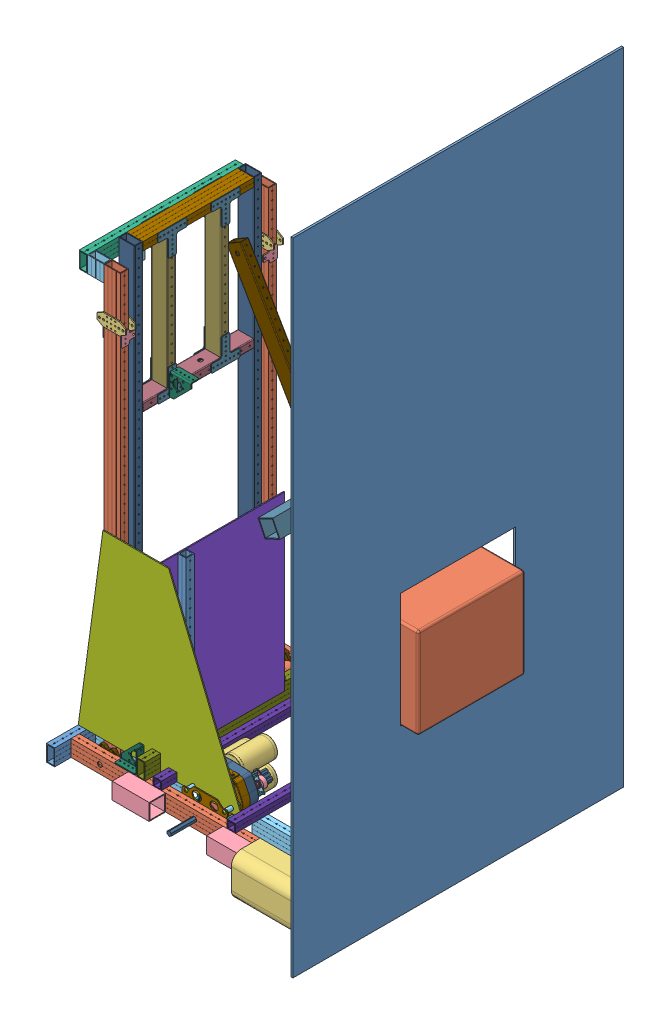
SolidWorks assembly Test Robot 3, configuration Default. Lengths in mm. (continued)
Components (placement in the parent): (continued)
- Elevator Drive Assembly-1: Elevator Drive Assembly [Default] at (512.9725 546.5466 390.8173) x (-1 0 0) z (0 0 1) size (95.12 72.01 584.2) (continued)
  - Hex Shaft Coupler-2: Hex Shaft Coupler [Default] at (253.5221 266.4359 300.4654) x (0.982439 -0.186583 0) z (0 0 -1) size (25.76 22.32 39.56) (continued)
    - 217-4008-002 Rev1_91251A108-7: 217-4008-002 Rev1_91251A108 [Default] at (9.7928 -7.025 -14.2875) x (-0.765668 0 0.643235) z (0 -1 0) size (4.65 4.65 12.51)
    - 217-4008-002 Rev1_91251A108-8: 217-4008-002 Rev1_91251A108 [Default] at (9.7928 -7.025 -4.7625) x (0.994016 0 0.109231) z (0 -1 0) size (4.65 4.65 12.51)
  - 12t Aluminum Hub Sprocket (35 Chain, 0.5 Hex Bore)-1: 12t Aluminum Hub Sprocket (35 Chain, 0.5 Hex Bore) [Default] at (253.5221 266.4359 340.2777) x (-0.856405 -0.516304 0) z (0 0 -1) size (40.29 40.29 10.67)
  - 217-2 Stage Versaplanetary STEP-3: 217-2 Stage Versaplanetary STEP [Default] at (253.5221 266.4359 467.3412) size (44.3 44.3 179.1)
    - 217-2625-001 Rev1-1: 217-2625-001 Rev1 [Default] at origin size (42 42 18)
    - 217-2625-002 Rev1-1: 217-2625-002 Rev1 [Default] at (0 0 -29.4) size (42 42 17.13)
    - 217-2625-003 Rev1-1: 217-2625-003 Rev1 [Default] at (0 0 -43.6478) x (1 0 0) z (0 0 -1) size (17 17 64.12)
    - 217-2625-009 Rev1-1: 217-2625-009 Rev1 [Default] at (0 0 -3.48) x (0 -1 0) z (0 0 -1) size (18 18 13)
    - 217-2816-001 Rev1-1: 217-2816-001 Rev1 [Default] at (0 0 -16.85) x (1 0 0) z (0 0 -1) size (42 42 14.5)
    - 217-2625-007 Rev1_Sun_Driver01-1: 217-2625-007 Rev1_Sun_Driver01 [Default] at (0 0 -11.767) x (0.055822 0.998441 0) z (0 0 1) size (14.49 14.49 12.72)
    - 217-2625-100-1: 217-2625-100 [Default] at (0 0 -18.467) x (0 1 0) z (0 0 1) size (39.26 38.9 12.7)
      - 217-2625-008 Rev1-1: 217-2625-008 Rev1 [Default] at origin size (34.7 34.7 4.7)
      - 217-2625-010 Rev1-1: 217-2625-010 Rev1 [Default] at (0 10.193 3.65) x (0.999813 0.019336 0) z (0 0 1) size (4 4 12)
      - 217-2625-010 Rev1-2: 217-2625-010 Rev1 [Default] at (8.691 -5.3258 3.65) size (4 4 12)
      - 217-2625-010 Rev1-3: 217-2625-010 Rev1 [Default] at (-8.691 -5.3258 3.65) size (4 4 12)
      - 217-2625-005 Rev1_Planet_Revolving_Follower01-1: 217-2625-005 Rev1_Planet_Revolving_Follower01 [Default] at (8.691 -5.3258 6.35) x (0.932816 0.360354 0) z (0 0 1) size (16.91 16.92 8)
      - 217-2625-005 Rev1_Planet_Revolving_Follower01-2: 217-2625-005 Rev1_Planet_Revolving_Follower01 [Default] at (-8.691 -5.3258 6.35) x (-0.932788 -0.360426 0) z (0 0 1) size (16.91 16.92 8)
      - 217-2625-005 Rev1_Planet_Revolving_Follower01-3: 217-2625-005 Rev1_Planet_Revolving_Follower01 [Default] at (0 10.193 6.35) x (0.893583 0.448898 0) z (0 0 1) size (16.91 16.92 8)
    - 217-2822-003 Rev4-1: 217-2822-003 Rev4 [Default] at (0 0 9) x (0 1 0) z (0 0 1) size (42 42 4.8)
    - 217-2625-011 Rev1-1: 217-2625-011 Rev1 [Default] at (0 0 1.37) x (1 0 0) z (0 -1 0) size (8.01 7.5 7.94)
    - SSA_SSA0832-0500ZC-1: SSA_SSA0832-0500ZC [Default] at (17.5 -17.5 10.5) x (0.189399 -0.9819 0) z (-0.9819 -0.189399 0) size (6.73 16.76 6.73)
    - 217-2742-1: 217-2742 [Default] at (0 0 -43.1002) x (0 0 1) z (-1 0 0) size (7 28 28)
    - 217-2742-2: 217-2742 [Default] at (0 0 -51.4002) x (0 0 1) z (-0.997393 0.072165 0) size (7 28 28)
    - SSA_SSA0832-1750ZC-1: SSA_SSA0832-1750ZC [Default] at (17.5 -17.5 -47.261) x (1 0 0) z (0 1 0) size (6.73 48.51 6.73)
    - SSA_SSA0832-1750ZC-2: SSA_SSA0832-1750ZC [Default] at (-17.5 17.5 -47.261) x (1 0 0) z (0 1 0) size (6.73 48.51 6.73)
    - 217-2625-018 Rev1_98541A410-1: 217-2625-018 Rev1_98541A410 [Default] at (0 0 -35.4954) x (0 0 -1) z (0.980859 -0.194721 0) size (1 19.6 17.4)
    - 217-2625-017 Rev1_9714K61-1: 217-2625-017 Rev1_9714K61 [Default] at (0 0 -44.1002) x (-0.695225 0.718792 0) z (-0.718792 -0.695225 0) size (28.51 4.98 30.18)
    - PINL-M020-006-S-1: PINL-M020-006-S [Default] at (-18.5 13.6657 -9.5) x (0 0 -1) z (1 0 0) size (6 2 2)
    - PINL-M020-006-S-2: PINL-M020-006-S [Default] at (-18.5 13.6657 -22.2) x (0 0 -1) z (0.23951 -0.970894 0) size (6 2 2)
    - 217-2816-001 Rev1-2: 217-2816-001 Rev1 [Default] at (0 0 -29.55) x (1 0 0) z (0 0 -1) size (42 42 14.5)
    - 217-3106-000 Rev2_NO SUN-1: 217-3106-000 Rev2_NO SUN [Default] at (0 0 -31.5454) size (40.34 37.58 17.71)
      - 217-3106-002 Rev1_Planet_Revolving_Follower01-1: 217-3106-002 Rev1_Planet_Revolving_Follower01 [Default] at (0 10.2965 6.35) x (0.979503 -0.20143 0) z (0 0 1) size (16.8 16.83 8)
      - 217-3106-003 Rev1-1: 217-3106-003 Rev1 [Default] at origin size (34.7 34.7 4.7)
      - 217-3106-001 Rev1_Sun_Driver01-1: 217-3106-001 Rev1_Sun_Driver01 [Default] at (0 0 9.0125) x (1 0 0) z (0 0 -1) size (14.56 14.56 12.7)
      - 217-3106-002 Rev1_Planet_Revolving_Follower01-2: 217-3106-002 Rev1_Planet_Revolving_Follower01 [Default] at (8.917 -5.1482 6.35) x (-0.664195 -0.74756 0) z (0 0 1) size (16.8 16.83 8)
      - 217-3106-002 Rev1_Planet_Revolving_Follower01-3: 217-3106-002 Rev1_Planet_Revolving_Follower01 [Default] at (-8.917 -5.1482 6.35) x (-0.315308 0.948989 0) z (0 0 1) size (16.8 16.83 8)
      - 217-2625-010 Rev1-1: 217-2625-010 Rev1 [Default] at (8.917 -5.1482 3.65) x (0.999617 0.027658 0) z (0 0 1) size (4 4 12)
      - 217-2625-010 Rev1-2: 217-2625-010 Rev1 [Default] at (-8.917 -5.1482 3.65) x (-0.475856 -0.879523 0) z (0 0 1) size (4 4 12)
      - 217-2625-010 Rev1-3: 217-2625-010 Rev1 [Default] at (0 10.2965 3.65) x (-0.523761 0.851865 0) z (0 0 1) size (4 4 12)
    - 775 pro-1: 775 pro [Default] at (0 0 10.5) x (0 0 1) z (-1 0 0) size (88 44.3 44.3)
  - Hex Shaft Coupler-3: Hex Shaft Coupler [Default] at (253.5221 266.4359 373.941) x (0.576903 -0.816813 0) z (0 0 -1) size (25.76 22.32 39.56)
    - 217-4008-001 Rev1-1: 217-4008-001 Rev1 [Default] at origin size (25.38 10.66 39.56)
    - 217-4008-001 Rev1-2: 217-4008-001 Rev1 [Default] x (1 0 0) z (0 0 -1) size (25.38 10.66 39.56)
    - 217-4008-002 Rev1_91251A108-1: 217-4008-002 Rev1_91251A108 [Default] at (9.7928 7.025 4.7625) x (0.994016 0 -0.109231) z (0 1 0) size (4.65 4.65 12.51)
    - 217-4008-002 Rev1_91251A108-2: 217-4008-002 Rev1_91251A108 [Default] at (9.7928 7.025 14.2875) x (-0.765668 0 -0.643235) z (0 1 0) size (4.65 4.65 12.51)
    - 217-4008-002 Rev1_91251A108-3: 217-4008-002 Rev1_91251A108 [Default] at (-9.7928 7.025 14.2875) x (-0.114094 0 0.99347) z (0 1 0) size (4.65 4.65 12.51)
    - 217-4008-002 Rev1_91251A108-4: 217-4008-002 Rev1_91251A108 [Default] at (-9.7928 7.025 4.7625) x (0.20346 0 0.979083) z (0 1 0) size (4.65 4.65 12.51)
    - 217-4008-002 Rev1_91251A108-5: 217-4008-002 Rev1_91251A108 [Default] at (-9.7928 -7.025 -4.7625) x (0.20346 0 -0.979083) z (0 -1 0) size (4.65 4.65 12.51)
    - 217-4008-002 Rev1_91251A108-6: 217-4008-002 Rev1_91251A108 [Default] at (-9.7928 -7.025 -14.2875) x (-0.114094 0 -0.99347) z (0 -1 0) size (4.65 4.65 12.51)
    - 217-4008-002 Rev1_91251A108-7: 217-4008-002 Rev1_91251A108 [Default] at (9.7928 -7.025 -14.2875) x (-0.765668 0 0.643235) z (0 -1 0) size (4.65 4.65 12.51)
    - 217-4008-002 Rev1_91251A108-8: 217-4008-002 Rev1_91251A108 [Default] at (9.7928 -7.025 -4.7625) x (0.994016 0 0.109231) z (0 -1 0) size (4.65 4.65 12.51)
  - VersaFrame Corner Gusset-1: VersaFrame Corner Gusset [Default] at (228.2491 291.8994 603.9032) x (0 -1 0) z (0 0 1) size (69.72 69.72 25.4)
  - VersaFrame Corner Gusset-2: VersaFrame Corner Gusset [Default] at (228.2491 291.8994 70.5032) x (1 0 0) z (0 0 -1) size (69.72 69.72 25.4)
- Elevator Bottom Shaft-1: Elevator Bottom Shaft [Default] at (109.0247 229.2599 486.7205) size (14.48 12.67 431.8)
- VersaFrame Face Bearing Mount-1: VersaFrame Face Bearing Mount [Default] at (132.1964 229.3742 537.5205) size (101.35 50.55 2.29)
- Intake Mechanism 2-1: Intake Mechanism 2 [Default] at (654.4226 630.6506 981.9417) x (0.923728 0.383049 0) z (0 0 -1) size (256.17 455.52 539.78)
  - Intake Arm-1: Intake Arm [Default] at (304.7258 -373.9972 -25.4788) x (0 0 -1) z (-0.383049 0.923728 0) size (25.4 25.4 482.6)
  - am-3480+4IN+500Hex+Bore+Compliant+Wheel-1: am-3480+4IN+500Hex+Bore+Compliant+Wheel [Default] at (239.3186 -68.108 -0.7547) x (0.383049 -0.923728 0) z (-0.923728 -0.383049 0) size (101.6 101.6 25.74)
    - 4IN Compliant Wheel FINAL Overmold-1: 4IN Compliant Wheel FINAL Overmold [Default] at (-16.2374 3.8509 18.652) size (101.6 101.6 25.74)
    - 2in Wheel Intergrated 0500 HEX Hub-1: 2in Wheel Intergrated 0500 HEX Hub [Default] at (-16.2374 3.8509 5.952) x (-1 0 0) z (0 0 -1) size (41.91 41.91 25.4)
  - VersaFrame Side Bearing Mount-1: VersaFrame Side Bearing Mount [Default] at (194.5184 -69.1075 3.0962) x (-0.383049 0.923728 0) z (-0.923728 -0.383049 0) size (63.5 61.91 2.29)
  - am-3480+4IN+500Hex+Bore+Compliant+Wheel-2: am-3480+4IN+500Hex+Bore+Compliant+Wheel [Default] at (180.2057 74.4434 11.6723) x (0.274302 -0.661484 0.697996) z (-0.923728 -0.383049 0) size (101.6 101.6 25.74)
    - 4IN Compliant Wheel FINAL Overmold-1: 4IN Compliant Wheel FINAL Overmold [Default] at (-16.2374 3.8509 18.652) size (101.6 101.6 25.74)
    - 2in Wheel Intergrated 0500 HEX Hub-1: 2in Wheel Intergrated 0500 HEX Hub [Default] at (-16.2374 3.8509 5.952) x (-1 0 0) z (0 0 -1) size (41.91 41.91 25.4)
  - VersaFrame Side Bearing Mount-2: VersaFrame Side Bearing Mount [Default] at (136.1417 71.6687 3.0962) x (-0.383049 0.923728 0) z (-0.923728 -0.383049 0) size (63.5 61.91 2.29)
  - VersaFrame Side Bearing Mount-3: VersaFrame Side Bearing Mount [Default] at (194.5184 -69.1075 403.1462) x (0.383049 -0.923728 0) z (-0.923728 -0.383049 0) size (63.5 61.91 2.29)
  - am-3480+4IN+500Hex+Bore+Compliant+Wheel-3: am-3480+4IN+500Hex+Bore+Compliant+Wheel [Default] at (179.6725 75.7295 392.5882) x (0.344557 -0.830905 -0.436896) z (-0.923728 -0.383049 0) size (101.6 101.6 25.74)
    - 4IN Compliant Wheel FINAL Overmold-1: 4IN Compliant Wheel FINAL Overmold [Default] at (-16.2374 3.8509 18.652) size (101.6 101.6 25.74)
    - 2in Wheel Intergrated 0500 HEX Hub-1: 2in Wheel Intergrated 0500 HEX Hub [Default] at (-16.2374 3.8509 5.952) x (-1 0 0) z (0 0 -1) size (41.91 41.91 25.4)
  - VersaFrame Side Bearing Mount-4: VersaFrame Side Bearing Mount [Default] at (136.1417 71.6687 403.1462) x (0.383049 -0.923728 0) z (-0.923728 -0.383049 0) size (63.5 61.91 2.29)
  - am-3480+4IN+500Hex+Bore+Compliant+Wheel-4: am-3480+4IN+500Hex+Bore+Compliant+Wheel [Default] at (226.7149 -37.714 403.9966) x (-0.376731 0.908492 -0.180877) z (-0.923728 -0.383049 0) size (101.6 101.6 25.74)
    - 4IN Compliant Wheel FINAL Overmold-1: 4IN Compliant Wheel FINAL Overmold [Default] at (-16.2374 3.8509 18.652) size (101.6 101.6 25.74)
    - 2in Wheel Intergrated 0500 HEX Hub-1: 2in Wheel Intergrated 0500 HEX Hub [Default] at (-16.2374 3.8509 5.952) x (-1 0 0) z (0 0 -1) size (41.91 41.91 25.4)
  - Intake Arm-2: Intake Arm [Default] at (304.7258 -373.9972 431.7212) x (0 0 -1) z (-0.383049 0.923728 0) size (25.4 25.4 482.6)
- Intake Upright 2-1: Intake Upright 2 [Default] at (792.7234 -367.6528 524.8205) x (0 0 -1) z (0 1 0) size (25.4 50.8 127)
- PowerUp Cube-1: PowerUp Cube [Default] at (995.8472 521.3472 943.9205) x (0 1 0) z (0 0 1) size (330.2 279.4 330.2) (hidden)
- Intake Upright 2-2: Intake Upright 2 [Default] at (843.5234 -418.4528 524.8205) x (0 0 -1) z (0 1 0) size (25.4 50.8 127) (hidden)
- Intake Upright 2-3: Intake Upright 2 [Default] at (119.5472 305.371 550.2205) x (0 0 -1) z (1 0 0) size (25.4 50.8 127) (hidden)
- Intake Mechanism 2-2: Intake Mechanism 2 [Default] at (667.1226 528.9744 956.5417) x (0.923728 0.383049 0) z (0 0 -1) size (256.17 455.52 539.78) (hidden)
  - Intake Arm-1: Intake Arm [Default] at (304.7258 -373.9972 -25.4788) x (0 0 -1) z (-0.383049 0.923728 0) size (25.4 25.4 482.6)
  - am-3480+4IN+500Hex+Bore+Compliant+Wheel-1: am-3480+4IN+500Hex+Bore+Compliant+Wheel [Default] at (239.3186 -68.108 -0.7547) x (0.383049 -0.923728 0) z (-0.923728 -0.383049 0) size (101.6 101.6 25.74)
    - 4IN Compliant Wheel FINAL Overmold-1: 4IN Compliant Wheel FINAL Overmold [Default] at (-16.2374 3.8509 18.652) size (101.6 101.6 25.74)
    - 2in Wheel Intergrated 0500 HEX Hub-1: 2in Wheel Intergrated 0500 HEX Hub [Default] at (-16.2374 3.8509 5.952) x (-1 0 0) z (0 0 -1) size (41.91 41.91 25.4)
  - VersaFrame Side Bearing Mount-1: VersaFrame Side Bearing Mount [Default] at (194.5184 -69.1075 3.0962) x (-0.383049 0.923728 0) z (-0.923728 -0.383049 0) size (63.5 61.91 2.29)
  - am-3480+4IN+500Hex+Bore+Compliant+Wheel-2: am-3480+4IN+500Hex+Bore+Compliant+Wheel [Default] at (180.2057 74.4434 11.6723) x (0.274302 -0.661484 0.697996) z (-0.923728 -0.383049 0) size (101.6 101.6 25.74)
    - 4IN Compliant Wheel FINAL Overmold-1: 4IN Compliant Wheel FINAL Overmold [Default] at (-16.2374 3.8509 18.652) size (101.6 101.6 25.74)
    - 2in Wheel Intergrated 0500 HEX Hub-1: 2in Wheel Intergrated 0500 HEX Hub [Default] at (-16.2374 3.8509 5.952) x (-1 0 0) z (0 0 -1) size (41.91 41.91 25.4)
  - VersaFrame Side Bearing Mount-2: VersaFrame Side Bearing Mount [Default] at (136.1417 71.6687 3.0962) x (-0.383049 0.923728 0) z (-0.923728 -0.383049 0) size (63.5 61.91 2.29)
  - VersaFrame Side Bearing Mount-3: VersaFrame Side Bearing Mount [Default] at (194.5184 -69.1075 403.1462) x (0.383049 -0.923728 0) z (-0.923728 -0.383049 0) size (63.5 61.91 2.29)
  - am-3480+4IN+500Hex+Bore+Compliant+Wheel-3: am-3480+4IN+500Hex+Bore+Compliant+Wheel [Default] at (179.6725 75.7295 392.5882) x (0.344557 -0.830905 -0.436896) z (-0.923728 -0.383049 0) size (101.6 101.6 25.74)
    - 4IN Compliant Wheel FINAL Overmold-1: 4IN Compliant Wheel FINAL Overmold [Default] at (-16.2374 3.8509 18.652) size (101.6 101.6 25.74)
    - 2in Wheel Intergrated 0500 HEX Hub-1: 2in Wheel Intergrated 0500 HEX Hub [Default] at (-16.2374 3.8509 5.952) x (-1 0 0) z (0 0 -1) size (41.91 41.91 25.4)
  - VersaFrame Side Bearing Mount-4: VersaFrame Side Bearing Mount [Default] at (136.1417 71.6687 403.1462) x (0.383049 -0.923728 0) z (-0.923728 -0.383049 0) size (63.5 61.91 2.29)
  - am-3480+4IN+500Hex+Bore+Compliant+Wheel-4: am-3480+4IN+500Hex+Bore+Compliant+Wheel [Default] at (226.7149 -37.714 403.9966) x (-0.376731 0.908492 -0.180877) z (-0.923728 -0.383049 0) size (101.6 101.6 25.74)
    - 4IN Compliant Wheel FINAL Overmold-1: 4IN Compliant Wheel FINAL Overmold [Default] at (-16.2374 3.8509 18.652) size (101.6 101.6 25.74)
    - 2in Wheel Intergrated 0500 HEX Hub-1: 2in Wheel Intergrated 0500 HEX Hub [Default] at (-16.2374 3.8509 5.952) x (-1 0 0) z (0 0 -1) size (41.91 41.91 25.4)
  - Intake Arm-2: Intake Arm [Default] at (304.7258 -373.9972 431.7212) x (0 0 -1) z (-0.383049 0.923728 0) size (25.4 25.4 482.6)
- PowerUp Cube-2: PowerUp Cube [Default] at (995.8472 330.771 931.2205) x (0 1 0) z (0 0 1) size (330.2 279.4 330.2) (hidden)
- Side support Panal with squirrel_Rev1-1: Side support Panal with squirrel_Rev1 [Default] at (489.9994 334.8792 486.7205) x (-1 0 0) z (0 0 -1) size (585.27 560.46 41.2) (hidden)
- Grasper-1: Grasper [Default] at (443.6962 299.0803 477.7436) x (0 0 1) z (0 1 0) size (203.2 338.44 449.25) (hidden)
  - Grasper Upright-1: Grasper Upright [Default] at (116.9269 192.6182 -294.9916) size (25.4 25.4 355.6)
  - Grasper Upright-2: Grasper Upright [Default] at (294.7269 192.6182 -294.9916) size (25.4 25.4 355.6)
  - Grasper Bottom-1: Grasper Bottom [Default] at (104.2269 155.6299 48.3477) x (0 1 0) z (1 0 0) size (203.2 127 203.2)
  - Grasper Top Support-1: Grasper Top Support [Default] at (142.3269 -408.5863 168.3294) x (1 0 0) z (0 0.910364 0.413808) size (25.4 25.4 152.4)
  - Grasper Top Support-2: Grasper Top Support [Default] at (269.3269 -408.5863 168.3294) x (1 0 0) z (0 0.910364 0.413808) size (25.4 25.4 152.4)
  - Grasper Top-1: Grasper Top [Default] at (282.0269 181.1993 446.3981) x (0 0.910364 0.413808) z (-1 0 0) size (203.2 177.8 152.4)
- PowerUp Cube-4: PowerUp Cube [Default] at (995.8472 800.7472 943.9205) x (-1 0 0) z (0 0 1) size (330.2 279.4 330.2) (hidden)
- Grasper 2 Top-1: Grasper 2 Top [Default] at (253.9381 1026.3764 368.8036) x (0.90402 0.42749 0) z (0.42749 -0.90402 0) size (332.74 355.6 230.23)
  - Grasper Top Support 2-1: Grasper Top Support 2 [Default] at (970.84 202.7529 145.7054) x (0.0049 0 0.999988) z (-0.999988 0 0.0049) size (25.4 25.4 279.4)
  - Grasper Top Support 2-2: Grasper Top Support 2 [Default] at (970.84 380.5529 145.7054) x (0.0049 0 0.999988) z (-0.999988 0 0.0049) size (25.4 25.4 279.4)
  - Grasper Cube Orientation Compensation Device-1: Grasper Cube Orientation Compensation Device [Default] at (170.8038 113.8529 160.6925) x (0.0049 0 0.999988) z (0 1 0) size (50.8 50.8 355.6)
  - Grasper 2 Kick Plate-1: Grasper 2 Kick Plate [Default] at (170.8118 367.8529 162.3253) x (0 -1 0) z (-0.999988 0 0.0049) size (152.4 203.2 2.54)
- Grasper 2 Bottom-1: Grasper 2 Bottom [Default] at (412.7936 1115.0952 364.1287) x (1 0 0) z (0 -1 0) size (265.11 205.49 406.4)
  - Grasper Upright 2-1: Grasper Upright 2 [Default] at (162.5578 232.8278 -253.9782) size (25.4 25.4 406.4)
  - Grasper Upright 2-2: Grasper Upright 2 [Default] at (162.5578 410.6278 -253.9782) size (25.4 25.4 406.4)
  - Grasper Bottom Support 2-1: Grasper Bottom Support 2 [Default] at (-370.8422 232.8278 482.6218) x (0 0 -1) z (1 0 0) size (25.4 25.4 203.2)
  - Grasper Bottom Support 2-2: Grasper Bottom Support 2 [Default] at (-370.8422 410.6278 482.6218) x (0 0 -1) z (1 0 0) size (25.4 25.4 203.2)
  - VersaFrame Side Bearing Mount-1: VersaFrame Side Bearing Mount [Default] at (133.9828 220.1278 412.7718) x (0 0 -1) z (0 -1 0) size (63.5 61.91 2.29)
- Elevator Arm Section 2-1: Elevator Arm Section 2 [Default] at (521.2647 746.2528 569.2705) x (0 0 1) z (-0.502198 0.864753 0) size (25.4 50.8 825.5)
- Grasper 3 Bottom-1: Grasper 3 Bottom [Default] at (574.3419 1161.5271 374.7469) x (0.883482 -0.468466 0) z (-0.468466 -0.883482 0) size (265.11 154.69 254) (hidden)
  - Grasper Bottom Support 2-1: Grasper Bottom Support 2 [Default] at (-314.0574 249.8956 488.4615) x (0 0 -1) z (1 0 0) size (25.4 25.4 203.2)
  - Grasper Bottom Support 2-2: Grasper Bottom Support 2 [Default] at (-314.0574 376.8956 488.4615) x (0 0 -1) z (1 0 0) size (25.4 25.4 203.2)
  - VersaFrame Side Bearing Mount-1: VersaFrame Side Bearing Mount [Default] at (190.7676 237.1956 418.6115) x (0 0 -1) z (0 -1 0) size (63.5 61.91 2.29)
  - Grasper 3 Bottom Upright-1: Grasper 3 Bottom Upright [Default] at (219.3426 249.8956 -248.1385) size (25.4 25.4 254)
  - Grasper 3 Bottom Upright-2: Grasper 3 Bottom Upright [Default] at (219.3426 376.8956 -248.1385) size (25.4 25.4 254)
- Grasper 3 Top-1: Grasper 3 Top [Default] at (582.2052 1181.1454 302.4184) x (0.999988 -0.0049 0) z (-0.0049 -0.999988 0) size (390.8 355.6 408.14) (hidden)
  - Grasper Top Support 2-1: Grasper Top Support 2 [Default] at (806.758 294.5381 163.7212) x (0.0049 0 0.999988) z (-0.999988 0 0.0049) size (25.4 25.4 279.4)
  - Grasper Top Support 2-2: Grasper Top Support 2 [Default] at (806.758 472.3381 163.7212) x (0.0049 0 0.999988) z (-0.999988 0 0.0049) size (25.4 25.4 279.4)
  - Grasper Cube Orientation Compensation Device-1: Grasper Cube Orientation Compensation Device [Default] at (6.7218 205.6381 178.7083) x (0.0049 0 0.999988) z (0 1 0) size (50.8 50.8 355.6)
  - VersaFrame Side Bearing Mount-1: VersaFrame Side Bearing Mount [Default] at (-33.0824 485.0381 478.9898) x (0.0049 0 0.999988) z (0 1 0) size (63.5 61.91 2.29)
  - Grasper Upright 2-1: Grasper Upright 2 [Default] at (-7.7745 472.3381 -187.8922) x (-0.999988 0 0.0049) z (0.0049 0 0.999988) size (25.4 25.4 406.4)
  - VersaFrame Side Bearing Mount-2: VersaFrame Side Bearing Mount [Default] at (-33.0824 281.8381 478.9898) x (-0.0049 0 -0.999988) z (0 -1 0) size (63.5 61.91 2.29)
  - Grasper Upright 2-2: Grasper Upright 2 [Default] at (-7.7745 294.5381 -187.8922) x (0.999988 0 -0.0049) z (0.0049 0 0.999988) size (25.4 25.4 406.4)
- Portal-1: Portal [Default] at (957.8234 153.0472 1216.9705) x (0 0 -1) z (1 0 0) size (1022.35 1981.2 6.35)
- PowerUp Cube-5: PowerUp Cube [Default] at (688.2049 661.0472 883.7225) size (330.2 279.4 330.2)
Mates (geometry in assembly coordinates):
- Coincident2: coincident aligned: plane of Test Base 3-1/Base Side Rail Internal-1 through (360.9234 203.8472 943.9205) normal (0 -1 0); plane of Elevator Base Frame-1/Elevator Fixed Frame-1 through (157.7234 203.8472 956.6205) normal (0 -1 0)
- Distance1: distance = 50.8 mm anti-aligned: plane of Elevator Base Frame-1/Elevator Fixed Frame-1 through (132.3234 1524.6472 943.9205) normal (-1 0 0); plane of Test Base 3-1/Base Rear Rail-1 through (81.5234 203.8472 1070.9205) normal (1 0 0)
- Coincident4: coincident anti-aligned: plane of Elevator Base Frame-1/Elevator Fixed Frame-1 through (132.3234 1524.6472 969.3205) normal (0 0 1); plane of Elevator Side Panels-1 through (132.3234 254.6472 969.3205) normal (0 0 -1)
- Coincident7: coincident anti-aligned: plane of Elevator Base Frame-1/Elevator Fixed Frame-2 through (132.3234 1524.6472 486.7205) normal (0 0 -1); plane of Elevator Side Panels-2 through (132.3234 254.6472 486.7205) normal (0 0 1)
- Coincident10: coincident anti-aligned: plane of Test Base 3-1/Base Side Rail Internal-1 through (360.9234 254.6472 943.9205) normal (0 1 0); plane of Elevator Side Panels-1 through (56.1234 254.6472 972.4955) normal (0 -1 0)
- Coincident11: coincident anti-aligned: plane of Test Base 3-1/Base Side Rail Internal-4 through (81.5234 254.6472 512.1205) normal (0 1 0); plane of Elevator Side Panels-2 through (56.1234 254.6472 486.7205) normal (0 -1 0)
- Coincident13: coincident aligned: plane of Test Base 3-1/Electronics Upright-1 through (322.8234 813.4472 905.8205) normal (0 1 0); plane of Electronics Panel-1 through (310.1234 813.4472 969.3205) normal (0 1 0)
- Coincident14: coincident anti-aligned: plane of Elevator Side Panels-1 through (132.3234 254.6472 969.3205) normal (0 0 -1); plane of Electronics Panel-1 through (310.1234 280.0472 969.3205) normal (0 0 1)
- Coincident20: coincident anti-aligned: plane of Test Base 3-1/Electronics Upright-2 through (310.1234 203.8472 537.5205) normal (-1 0 0); plane of Electronics Panel-1 through (310.1234 280.0472 969.3205) normal (1 0 0)
- Coincident46: coincident aligned: plane of Test Base 3-1/Base Rear Rail-1 through (56.1234 203.8472 1070.9205) normal (0 -1 0); plane of Elevator Base Frame-1/Elevator Fixed Frame-1 through (157.7234 203.8472 956.6205) normal (0 -1 0)
- Coincident57: coincident anti-aligned: plane of Test Base 3-1/Base Side Rail Internal-1 through (360.9234 203.8472 943.9205) normal (0 0 1); plane of Elevator Base Frame-1/Elevator Fixed Frame-1 through (132.3234 1524.6472 943.9205) normal (0 0 -1)
- Distance27: distance = 19.05 mm anti-aligned: plane of Elevator Moving Stage-2/Elevator Moving Stage Upright-1 through (134.8634 1575.4472 531.1705) normal (0 0 -1); plane of Elevator Base Frame-1/Elevator Fixed Frame-2 through (132.3234 1524.6472 512.1205) normal (0 0 1)
- Coincident58: coincident aligned: plane of Elevator Base Frame-1/Elevator Fixed Frame-2 through (132.3234 1524.6472 486.7205) normal (-1 0 0); plane of Elevator Moving Stage-2/Elevator Moving Stage Upright-1 through (132.3234 1575.4472 533.7105) normal (-1 0 0)
- Coincident60: coincident aligned: plane of Test Base 3-1/Base Side Rail-1 through (81.5234 203.8472 1020.1205) normal (0 0 1); plane of Elevator Drive Assembly-1/Elevator Drive Assembly Base Rail-1 through (297.4234 280.0472 1020.1205) normal (0 0 1)
- Coincident61: coincident anti-aligned: plane of Test Base 3-1/Base Side Rail Internal-4 through (81.5234 203.8472 537.5205) normal (0 0 1); plane of VersaFrame Face Bearing Mount-1 through (81.5234 204.1012 537.5205) normal (0 0 -1)
- Coincident62: coincident aligned: plane of Test Base 3-1/Base Side Rail Internal-4 through (81.5234 254.6472 512.1205) normal (0 1 0); plane of VersaFrame Face Bearing Mount-1 through (81.5234 254.6472 539.8065) normal (0 1 0)
- Coincident63: coincident anti-aligned: plane of Test Base 3-1/Base Rear Rail-1 through (81.5234 203.8472 1070.9205) normal (1 0 0); plane of VersaFrame Face Bearing Mount-1 through (81.5234 254.6472 539.8065) normal (-1 0 0)
- Coincident64: coincident aligned: plane of Test Base 3-1/Base Side Rail Internal-4 through (81.5234 203.8472 512.1205) normal (0 0 -1); plane of Elevator Bottom Shaft-1 through (109.0247 229.2599 512.1205) normal (0 0 -1)
- Distance29: distance = 19.05 mm aligned: plane of Elevator Bottom Shaft-1 through (112.6835 235.5972 943.9205) normal (0 1 0); plane of Test Base 3-1/Base Rear Rail-1 through (56.1234 254.6472 1070.9205) normal (0 1 0)
- Coincident65: coincident anti-aligned: plane of Test Base 3-1/Base Side Rail Internal-1 through (360.9234 254.6472 943.9205) normal (0 1 0); plane of Elevator Drive Assembly-1/Elevator Drive Assembly Base Rail-1 through (310.1234 254.6472 1020.1205) normal (0 -1 0)
- Coincident68: coincident aligned: plane of Test Base 3-1/Base Side Rail Internal-5 through (843.5234 203.8472 537.5205) normal (0 0 1); plane of Intake Upright 2-1 through (792.7234 -367.6528 537.5205) normal (0 0 1)
- Coincident69: coincident anti-aligned: plane of Test Base 3-1/Base Side Rail Internal-5 through (843.5234 254.6472 537.5205) normal (0 1 0); plane of Intake Upright 2-1 through (792.7234 254.6472 524.8205) normal (0 -1 0)
- Distance32: distance = 50.8 mm aligned: plane of Intake Upright 2-1 through (818.1234 381.6472 537.5205) normal (1 0 0); plane of Test Base 3-1/Base Rear Rail-2 through (868.9234 203.8472 1070.9205) normal (1 0 0)
- Coincident70: coincident anti-aligned: plane of Intake Mechanism 2-1/Intake Arm-2 through (805.3472 343.5472 537.5205) normal (0 0 -1); plane of Intake Upright 2-1 through (792.7234 -367.6528 537.5205) normal (0 0 1)
- Concentric10: concentric anti-aligned: cylinder of Intake Mechanism 2-1/Intake Arm-2 through (792.6472 356.2472 537.5205) axis (0 0 1) radius 2.0701; cylinder of Intake Upright 2-1 through (792.6472 356.2472 537.5205) axis (0 0 -1) radius 6.35
- Distance33: distance = 190.5 mm aligned: plane of PowerUp Cube-1 through (995.8472 521.3472 943.9205) normal (1 0 0); plane of Intake Mechanism 2-1/Intake Arm-1 through (805.3472 343.5472 994.7205) normal (1 0 0)
- Distance34: distance = 50.8 mm anti-aligned: plane of PowerUp Cube-1 through (716.4472 521.3472 613.7205) normal (0 0 -1); plane of Intake Mechanism 2-1/Intake Arm-2 through (805.3472 343.5472 562.9205) normal (0 0 1)
- LimitAngle1: limit planar angle = 1.570796 rad aligned: plane of Intake Mechanism 2-1/Intake Arm-1 through (779.9472 343.5472 994.7205) normal (-1 0 0); plane of Test Base 3-1/Base Front Rail-1 through (843.5234 254.6472 1070.9205) normal (0 1 0)
- Distance35: distance = 25.4 mm aligned: plane of PowerUp Cube-1 through (716.4472 851.5472 943.9205) normal (0 1 0); plane of Intake Mechanism 2-1/Intake Arm-1 through (792.6472 826.1472 1007.4205) normal (0 1 0)
- Coincident72: coincident aligned: plane of Test Base 3-1/Base Rear Rail-2 through (868.9234 203.8472 1070.9205) normal (1 0 0); plane of Intake Upright 2-2 through (868.9234 330.8472 537.5205) normal (1 0 0)
- Coincident73: coincident aligned: plane of Test Base 3-1/Base Side Rail Internal-5 through (843.5234 203.8472 537.5205) normal (0 0 1); plane of Intake Upright 2-2 through (843.5234 -418.4528 537.5205) normal (0 0 1)
- Coincident74: coincident aligned: plane of Test Base 3-1/Base Rear Rail-2 through (843.5234 203.8472 1070.9205) normal (0 -1 0); plane of Intake Upright 2-2 through (843.5234 203.8472 524.8205) normal (0 -1 0)
- Concentric12: concentric aligned: cylinder of Intake Upright 2-2 through (843.4472 305.4472 537.5205) axis (0 0 -1) radius 6.35; cylinder of Intake Upright 2-3 through (843.4472 305.4472 562.9205) axis (0 0 -1) radius 6.35
- Coincident75: coincident anti-aligned: plane of Intake Upright 2-2 through (843.5234 -418.4528 537.5205) normal (0 0 1); plane of Intake Upright 2-3 through (119.5472 305.371 537.5205) normal (0 0 -1)
- Coincident76: coincident anti-aligned: plane of Intake Upright 2-3 through (119.5472 305.371 537.5205) normal (0 0 -1); plane of Intake Mechanism 2-2/Intake Arm-2 through (818.0472 241.871 537.5205) normal (0 0 1)
- Distance38: distance = 50.8 mm aligned: plane of Intake Upright 2-3 through (741.8472 305.371 550.2205) normal (-1 0 0); plane of Intake Mechanism 2-2/Intake Arm-2 through (792.6472 241.871 512.1205) normal (-1 0 0)
- LimitAngle2: limit planar angle = 4.712389 rad anti-aligned: plane of Intake Upright 2-3 through (868.8472 279.971 562.9205) normal (0 -1 0); plane of Test Base 3-1/Base Rear Rail-2 through (843.5234 203.8472 1070.9205) normal (-1 0 0)
- Distance37: distance = 38.1 mm aligned: plane of Intake Upright 2-3 through (868.8472 279.971 562.9205) normal (0 -1 0); plane of Intake Mechanism 2-2/Intake Arm-2 through (805.3472 241.871 524.8205) normal (0 -1 0)
- Distance39: distance = 63.5 mm anti-aligned: plane of PowerUp Cube-2 through (716.4472 330.771 601.0205) normal (0 0 -1); plane of Intake Mechanism 2-2/Intake Arm-2 through (818.0472 241.871 537.5205) normal (0 0 1)
- Distance41: distance = 177.8 mm aligned: plane of PowerUp Cube-2 through (995.8472 330.771 931.2205) normal (1 0 0); plane of Intake Mechanism 2-2/Intake Arm-1 through (818.0472 241.871 969.3205) normal (1 0 0)
- Distance42: distance = 63.5 mm aligned: plane of PowerUp Cube-2 through (716.4472 660.971 931.2205) normal (0 1 0); plane of Intake Mechanism 2-2/Intake Arm-1 through (805.3472 724.471 982.0205) normal (0 1 0)
- Coincident77: coincident anti-aligned: plane of Elevator Base Frame-1/Elevator Fixed Frame-2 through (132.3234 1524.6472 486.7205) normal (0 0 -1); plane of Side support Panal with squirrel_Rev1-1 through (489.9994 334.8792 486.7205) normal (0 0 1)
- Angle1: planar angle = 0 rad aligned: plane of Test Base 3-1/Base Side Rail-2 through (81.5234 254.6472 435.9205) normal (0 1 0); plane of Side support Panal with squirrel_Rev1-1 through (489.9994 813.8246 486.7205) normal (0 1 0)
- Coincident78: coincident: plane of Elevator Base Frame-1/Elevator Fixed Frame-2 through (132.3234 1524.6472 486.7205) normal (-1 0 0); line of Side support Panal with squirrel_Rev1-1 through (132.3234 813.8246 484.1805) axis (0 0 1)
- Angle2: planar angle = 0 rad aligned: plane of Grasper-1/Grasper Upright-1 through (649.0144 753.3887 581.9705) normal (1 0 0); plane of Elevator Base Frame-1/Elevator Fixed Frame-1 through (183.1234 1524.6472 943.9205) normal (1 0 0)
- Coincident81: coincident aligned: plane of PowerUp Cube-1 through (716.4472 521.3472 613.7205) normal (0 0 -1); plane of PowerUp Cube-4 through (995.8472 521.3472 613.7205) normal (0 0 -1)
- Coincident82: coincident aligned: plane of PowerUp Cube-1 through (716.4472 521.3472 943.9205) normal (0 -1 0); plane of PowerUp Cube-4 through (995.8472 521.3472 943.9205) normal (0 -1 0)
- Coincident83: coincident aligned: plane of PowerUp Cube-1 through (995.8472 521.3472 943.9205) normal (1 0 0); plane of PowerUp Cube-4 through (995.8472 521.3472 943.9205) normal (1 0 0)
- Coincident84: coincident anti-aligned: plane of Grasper 2 Top-1/Grasper Top Support 2-2 through (513.6915 995.2103 762.0565) normal (0 0 1); plane of Grasper 2 Bottom-1/Grasper Upright 2-2 through (565.1914 619.7734 762.0565) normal (0 0 -1)
- Angle4: planar angle = 0 rad aligned: plane of Grasper 2 Bottom-1/Grasper Upright 2-2 through (588.0514 619.7734 764.5965) normal (1 0 0); plane of Test Base 3-1/Electronics Upright-2 through (335.5234 203.8472 537.5205) normal (1 0 0)
- Concentric23: concentric anti-aligned: cylinder of Grasper 2 Bottom-1/VersaFrame Side Bearing Mount-1 through (546.7764 702.3234 581.9705) axis (0 0 1) radius 14.2875; cylinder of Elevator Arm Section 2-1 through (546.7764 702.3234 581.9705) axis (0 0 -1) radius 6.35
- Concentric24: concentric aligned: cylinder of Elevator Moving Stage-2/Elevator Moving Stage Upright-1 through (157.7234 1372.2472 556.5705) axis (0 0 -1) radius 6.35; cylinder of Elevator Arm Section 2-1 through (157.7234 1372.2472 581.9705) axis (0 0 -1) radius 6.35
- Coincident88: coincident anti-aligned: plane of Elevator Moving Stage-2/Elevator Moving Stage Upright-1 through (134.8634 1575.4472 556.5705) normal (0 0 1); plane of Elevator Arm Section 2-1 through (125.1993 1382.7316 556.5705) normal (0 0 -1)
- Coincident89: coincident anti-aligned: plane of Grasper 2 Bottom-1/VersaFrame Side Bearing Mount-1 through (588.0514 734.0734 581.9705) normal (0 0 -1); plane of Elevator Arm Section 2-1 through (125.1993 1382.7316 581.9705) normal (0 0 1)
- Coincident93: coincident anti-aligned: plane of Test Base 3-1/Electronics Upright-1 through (310.1234 203.8472 893.1205) normal (-1 0 0); plane of Elevator Drive Assembly-1/Elevator Drive Assembly Base Rail-1 through (310.1234 305.4472 1020.1205) normal (1 0 0)
- Concentric25: concentric aligned: cylinder of Grasper 3 Bottom-1/VersaFrame Side Bearing Mount-1 through (546.7764 702.3234 609.6565) axis (0 0 1) radius 14.2875; cylinder of Grasper 3 Top-1/VersaFrame Side Bearing Mount-2 through (546.7764 702.3234 581.9705) axis (0 0 1) radius 14.2875
- Coincident94: coincident anti-aligned: plane of ? through (628.1478 482.8338 762.0565) normal (0 0 1); plane of Grasper 3 Top-1/Grasper Upright 2-1 through (648.6707 482.8788 762.0565) normal (0 0 -1)
- Concentric26: concentric anti-aligned: cylinder of Elevator Arm Section 2-1 through (546.7764 702.3234 581.9705) axis (0 0 -1) radius 6.35; cylinder of Grasper 3 Top-1/VersaFrame Side Bearing Mount-2 through (546.7764 702.3234 581.9705) axis (0 0 1) radius 14.2875
- Angle5: planar angle = 0 rad aligned: plane of Elevator Base Frame-1/Elevator Fixed Frame-2 through (183.1234 1524.6472 486.7205) normal (1 0 0); plane of Grasper 3 Top-1/Grasper Upright 2-2 through (588.0514 619.7734 586.7965) normal (1 0 0)
- Coincident96: coincident anti-aligned: plane of Elevator Arm Section 2-1 through (125.1993 1382.7316 581.9705) normal (0 0 1); plane of Grasper 3 Top-1/VersaFrame Side Bearing Mount-2 through (588.0514 734.0734 581.9705) normal (0 0 -1)
- Distance43: distance = 50.8 mm aligned: plane of Elevator Moving Stage-2/Elevator Crossbar-2 through (157.7234 1575.4472 150.1705) normal (0 1 0); plane of Elevator Base Frame-1/Elevator Fixed Frame Upper Crossbar-1 through (56.1234 1524.6472 969.3205) normal (0 1 0)
- Concentric27: concentric aligned: cylinder of Grasper 2 Top-1/Grasper Top Support 2-1 through (575.3514 1013.4734 558.8565) axis (0 0 1) radius 2.0701; cylinder of Grasper 2 Bottom-1/Grasper Upright 2-1 through (575.3514 1013.4734 584.2565) axis (0 0 1) radius 2.0701
- Coincident97: coincident anti-aligned: plane of Grasper 3 Bottom-1/VersaFrame Side Bearing Mount-1 through (598.1159 711.038 609.6565) normal (0 0 -1); plane of Grasper 3 Top-1/Grasper Upright 2-2 through (565.1914 619.7734 609.6565) normal (0 0 1)
- Coincident98: coincident anti-aligned: plane of Test Base 3-1/Blue Bumper-2 through (957.8234 330.8472 296.2205) normal (1 0 0); plane of Portal-1 through (957.8234 153.0472 1216.9705) normal (-1 0 0)
- Distance45: distance = 101.6 mm aligned: plane of Test Base 3-1/Blue Bumper-2 through (957.8234 330.8472 296.2205) normal (0 0 -1); plane of Portal-1 through (964.1734 153.0472 194.6205) normal (0 0 -1)
- Distance44: distance = 50.8 mm aligned: plane of Test Base 3-1/Blue Bumper-1 through (957.8234 203.8472 1159.8205) normal (0 -1 0); plane of Portal-1 through (964.1734 153.0472 1216.9705) normal (0 -1 0)
- Coincident100: coincident anti-aligned: plane of Portal-1 through (964.1734 661.0472 883.7225) normal (0 1 0); plane of PowerUp Cube-5 through (688.2049 661.0472 883.7225) normal (0 -1 0)
- Distance46: distance = 25.4 mm anti-aligned: plane of Portal-1 through (964.1734 1016.6472 528.1225) normal (0 0 1); plane of PowerUp Cube-5 through (688.2049 940.4472 553.5225) normal (0 0 -1)
